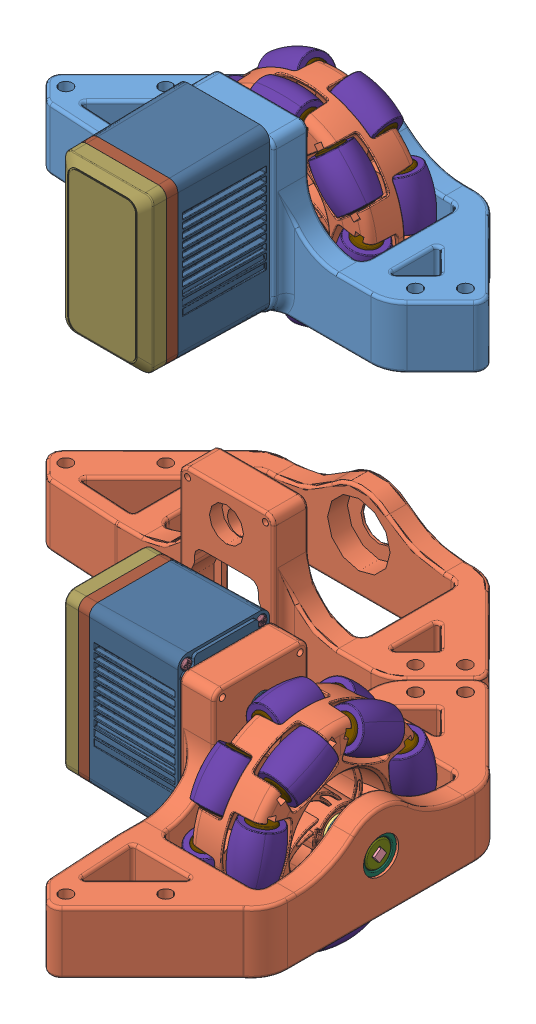
SolidWorks assembly holo_bracket_v4_Front_testfit, configuration Default. Lengths in mm.
Overall size (299.11 89.8 299.11).
176 component instances, 23 part files, 31 mates.
Components (placement in the parent):
- holo_bracket_v4_Left-1: holo_bracket_v4_Left [Default] at (46.7387 84.3688 112.9136) size (147.75 57.17 55.6)
- holo_bracket_v4_Right-1: holo_bracket_v4_Right [Default] at (163.9131 84.3688 230.088) size (181.94 57.17 181.94)
- V5 Smart Motor (276-4840) no cap-1: V5 Smart Motor (276-4840) no cap [Default] at (195.0559 116.1188 308.4808) x (0 -1 0) z (1 0 0) size (59.01 35.33 59.91)
  - V5 Smart Motor (276-4840).step-1: V5 Smart Motor (276-4840).step [Default] at origin size (59.01 35.33 59.91)
    - 276-4840-900 Rev6_Instruction.step-1: 276-4840-900 Rev6_Instruction.step [Default] at (-14.3 0 -17.2) size (52.79 15.94 38.15)
      - 276-4840-901 Rev6.step-1: 276-4840-901 Rev6.step [Default] at (10.75 -10.05 17.8) x (-1 0 0) z (0 0 1) size (49.9 1.6 38.15)
      - 276-4840-902 Rev2.step-1: 276-4840-902 Rev2.step [Default] at (31.25 -9.25 6.2) x (0 0 -1) z (0 -1 0) size (10.35 11.39 15.94)
      - 276-4840-022 Rev4.step-1: 276-4840-022 Rev4.step [Default] at (31.25 -9.25 6.2) x (0 0 -1) z (1 0 0) size (10.26 9.1 5.51)
    - 276-4840-110 Rev10_Instruction.step-1: 276-4840-110 Rev10_Instruction.step [Default] at (12.7 0 14.7) size (35.33 35.33 31.1)
      - 276-4840-061 Rev7_Ring_Gear_Fixed01 .6 Rev3.step-1: 276-4840-061 Rev7_Ring_Gear_Fixed01 .6 Rev3.step [Default] at origin size (28.79 28.39 24.6)
      - 276-4840-018 Rev6.step-1: 276-4840-018 Rev6.step [Default] at (0 0 6.7) x (-0.483174 0.875524 0) z (0 0 1) size (26 26 12.3)
      - 276-4840-059 Rev2.step-1: 276-4840-059 Rev2.step [Default] at (0 0 10.3) size (28.4 28.4 8.5)
      - 276-4840-062 Rev1.step-1: 276-4840-062 Rev1.step [Default] at (-12.1353 8.8168 12.3) x (0.956835 -0.290632 0) z (-0.290632 -0.956835 0) size (3.2 6.56 3.2)
      - 276-4840-062 Rev1.step-2: 276-4840-062 Rev1.step [Default] at (12.1353 8.8168 12.3) x (0.978427 0.206591 0) z (0.206591 -0.978427 0) size (3.2 6.56 3.2)
      - 276-4840-062 Rev1.step-3: 276-4840-062 Rev1.step [Default] at (-12.1353 -8.8168 12.3) x (0.72563 0.688086 0) z (0.688086 -0.72563 0) size (3.2 6.56 3.2)
    - 276-4840-001 Rev38.step-1: 276-4840-001 Rev38.step [Default] at origin size (57.3 33 46.9)
    - 276-4840-005 Rev27.step-1: 276-4840-005 Rev27.step [Default] at (0 0 -17.95) size (56.17 31.87 12.9)
    - 276-4840-004 Rev16.step-1: 276-4840-004 Rev16.step [Default] at (0 0 -19.2) size (56.01 31.71 9.21)
    - 276-4840-009 Rev3.step-1: 276-4840-009 Rev3.step [Default] at (25.45 13.5 15.7) x (0.19987 -0.979823 0) z (-0.979823 -0.19987 0) size (3.4 41.31 4.34)
    - 276-4840-009 Rev3.step-2: 276-4840-009 Rev3.step [Default] at (-25.45 -13.5 15.7) x (-0.998855 0.047836 0) z (0.047836 0.998855 0) size (3.4 41.31 4.34)
    - 276-4840-009 Rev3.step-3: 276-4840-009 Rev3.step [Default] at (25.45 -13.5 15.7) x (-0.975374 0.220559 0) z (0.220559 0.975374 0) size (3.4 41.31 4.34)
    - 276-4840-009 Rev3.step-4: 276-4840-009 Rev3.step [Default] at (-25.45 13.5 15.7) x (-0.922256 0.38658 0) z (0.38658 0.922256 0) size (3.4 41.31 4.34)
    - 276-4840-025 Rev19.step-1: 276-4840-025 Rev19.step [Default] at (12.7 0 -22.63) x (-0.993315 0.115437 0) z (0 0 1) size (14.82 14.83 35.18)
- V5 Smart Motor (276-4840) no cap-2: V5 Smart Motor (276-4840) no cap [Default] at (46.7387 116.1188 160.1636) x (0 -1 0) z (0 0 -1) size (59.01 35.33 59.91)
  - V5 Smart Motor (276-4840).step-1: V5 Smart Motor (276-4840).step [Default] at origin size (59.01 35.33 59.91)
    - 276-4840-900 Rev6_Instruction.step-1: 276-4840-900 Rev6_Instruction.step [Default] at (-14.3 0 -17.2) size (52.79 15.94 38.15)
      - 276-4840-901 Rev6.step-1: 276-4840-901 Rev6.step [Default] at (10.75 -10.05 17.8) x (-1 0 0) z (0 0 1) size (49.9 1.6 38.15)
      - 276-4840-902 Rev2.step-1: 276-4840-902 Rev2.step [Default] at (31.25 -9.25 6.2) x (0 0 -1) z (0 -1 0) size (10.35 11.39 15.94)
      - 276-4840-022 Rev4.step-1: 276-4840-022 Rev4.step [Default] at (31.25 -9.25 6.2) x (0 0 -1) z (1 0 0) size (10.26 9.1 5.51)
    - 276-4840-110 Rev10_Instruction.step-1: 276-4840-110 Rev10_Instruction.step [Default] at (12.7 0 14.7) size (35.33 35.33 31.1)
      - 276-4840-061 Rev7_Ring_Gear_Fixed01 .6 Rev3.step-1: 276-4840-061 Rev7_Ring_Gear_Fixed01 .6 Rev3.step [Default] at origin size (28.79 28.39 24.6)
      - 276-4840-018 Rev6.step-1: 276-4840-018 Rev6.step [Default] at (0 0 6.7) x (-0.483174 0.875524 0) z (0 0 1) size (26 26 12.3)
      - 276-4840-059 Rev2.step-1: 276-4840-059 Rev2.step [Default] at (0 0 10.3) size (28.4 28.4 8.5)
      - 276-4840-062 Rev1.step-1: 276-4840-062 Rev1.step [Default] at (-12.1353 8.8168 12.3) x (0.956835 -0.290632 0) z (-0.290632 -0.956835 0) size (3.2 6.56 3.2)
      - 276-4840-062 Rev1.step-2: 276-4840-062 Rev1.step [Default] at (12.1353 8.8168 12.3) x (0.978427 0.206591 0) z (0.206591 -0.978427 0) size (3.2 6.56 3.2)
      - 276-4840-062 Rev1.step-3: 276-4840-062 Rev1.step [Default] at (-12.1353 -8.8168 12.3) x (0.72563 0.688086 0) z (0.688086 -0.72563 0) size (3.2 6.56 3.2)
    - 276-4840-001 Rev38.step-1: 276-4840-001 Rev38.step [Default] at origin size (57.3 33 46.9)
    - 276-4840-005 Rev27.step-1: 276-4840-005 Rev27.step [Default] at (0 0 -17.95) size (56.17 31.87 12.9)
    - 276-4840-004 Rev16.step-1: 276-4840-004 Rev16.step [Default] at (0 0 -19.2) size (56.01 31.71 9.21)
    - 276-4840-009 Rev3.step-1: 276-4840-009 Rev3.step [Default] at (25.45 13.5 15.7) x (0.19987 -0.979823 0) z (-0.979823 -0.19987 0) size (3.4 41.31 4.34)
    - 276-4840-009 Rev3.step-2: 276-4840-009 Rev3.step [Default] at (-25.45 -13.5 15.7) x (-0.998855 0.047836 0) z (0.047836 0.998855 0) size (3.4 41.31 4.34)
    - 276-4840-009 Rev3.step-3: 276-4840-009 Rev3.step [Default] at (25.45 -13.5 15.7) x (-0.975374 0.220559 0) z (0.220559 0.975374 0) size (3.4 41.31 4.34)
    - 276-4840-009 Rev3.step-4: 276-4840-009 Rev3.step [Default] at (-25.45 13.5 15.7) x (-0.922256 0.38658 0) z (0.38658 0.922256 0) size (3.4 41.31 4.34)
    - 276-4840-025 Rev19.step-1: 276-4840-025 Rev19.step [Default] at (12.7 0 -22.63) x (-0.993315 0.115437 0) z (0 0 1) size (14.82 14.83 35.18)
- 0.375_ ID x 0.875_ OD x 0.281_ WD (Radial Bearing) (217-3239)-1: 0.375_ ID x 0.875_ OD x 0.281_ WD (Radial Bearing) (217-3239) [Default] at (259.8559 103.4188 308.4808) size (7.14 22.23 22.23)
- 0.375_ ID x 0.875_ OD x 0.281_ WD (Radial Bearing) (217-3239)-2: 0.375_ ID x 0.875_ OD x 0.281_ WD (Radial Bearing) (217-3239) [Default] at (46.7387 103.4188 88.2262) x (0 0 1) z (-1 0 0) size (7.14 22.23 22.23)
- 0.375in_ID_Bearing_Insert-1: 0.375in_ID_Bearing_Insert [Default] at (266.9999 103.4188 308.4808) x (0 0.801872 0.597496) z (-1 0 0) size (9.4 9.4 7.14)
- 0.375in_ID_Bearing_Insert-2: 0.375in_ID_Bearing_Insert [Default] at (46.7387 103.4188 95.3702) x (-0.877149 0.480218 0) z (0 0 -1) size (9.4 9.4 7.14)
- 2.75 Omni with inserts (276-1902) -1: 2.75 Omni with inserts (276-1902)  [Default] at (310.5892 53.5782 282.6771) x (0 0 1) z (-1 0 0) size (87.15 87.98 47.75)
  - 2.75 Omni-Directional Wheel - Double Roller (276-1902) -1: 2.75 Omni-Directional Wheel - Double Roller (276-1902)  [Default] at (25.8037 49.8406 68.5807) size (87.15 87.98 47.75)
    - 2.75 Omni-Directional Wheel - Double Roller (276-1902) .step-1: 2.75 Omni-Directional Wheel - Double Roller (276-1902) .step [Default] at origin size (87.15 87.98 47.75)
      - 276-1902-010 Rev1.step-1: 276-1902-010 Rev1.step [Default] at (0 27.5 8) x (1 0 0) z (0 0.828233 0.560383) size (23 27.81 20.35)
        - 276-1902-011 Rev1.step-1: 276-1902-011 Rev1.step [Default] at (0 -6.325 -26.7627) x (1 0 0) z (0 -0.973191 0.23) size (16.5 15 25.03)
        - 276-1902-012 Rev1.step-1: 276-1902-012 Rev1.step [Default] at origin size (17.5 10.34 18.34)
        - 276-1902-003 Rev1.step-1: 276-1902-003 Rev1.step [Default] x (0 -0.928523 0.371275) z (1 0 0) size (2 2 23)
      - 276-1902-010 Rev1.step-2: 276-1902-010 Rev1.step [Default] at (0 -27.5 -8) x (1 0 0) z (0 0.410464 0.911877) size (23 27.81 20.35)
        - 276-1902-011 Rev1.step-1: 276-1902-011 Rev1.step [Default] at (0 -6.325 -26.7627) x (1 0 0) z (0 -0.973191 0.23) size (16.5 15 25.03)
        - 276-1902-012 Rev1.step-1: 276-1902-012 Rev1.step [Default] at origin size (17.5 10.34 18.34)
        - 276-1902-003 Rev1.step-1: 276-1902-003 Rev1.step [Default] x (0 -0.928523 0.371275) z (1 0 0) size (2 2 23)
      - 276-1902-010 Rev1.step-3: 276-1902-010 Rev1.step [Default] at (-21.5004 -17.146 -8) x (0.62349 -0.781831 0) z (0.320913 0.25592 0.911877) size (23 27.81 20.35)
        - 276-1902-011 Rev1.step-1: 276-1902-011 Rev1.step [Default] at (0 -6.325 -26.7627) x (1 0 0) z (0 -0.973191 0.23) size (16.5 15 25.03)
        - 276-1902-012 Rev1.step-1: 276-1902-012 Rev1.step [Default] at origin size (17.5 10.34 18.34)
        - 276-1902-003 Rev1.step-1: 276-1902-003 Rev1.step [Default] x (0 -0.928523 0.371275) z (1 0 0) size (2 2 23)
      - 276-1902-010 Rev1.step-4: 276-1902-010 Rev1.step [Default] at (-26.8105 6.1193 -8) x (-0.222521 -0.974928 0) z (0.400172 -0.091337 0.911877) size (23 27.81 20.35)
        - 276-1902-011 Rev1.step-1: 276-1902-011 Rev1.step [Default] at (0 -6.325 -26.7627) x (1 0 0) z (0 -0.973191 0.23) size (16.5 15 25.03)
        - 276-1902-012 Rev1.step-1: 276-1902-012 Rev1.step [Default] at origin size (17.5 10.34 18.34)
        - 276-1902-003 Rev1.step-1: 276-1902-003 Rev1.step [Default] x (0 -0.928523 0.371275) z (1 0 0) size (2 2 23)
      - 276-1902-010 Rev1.step-5: 276-1902-010 Rev1.step [Default] at (-11.9318 24.7766 -8) x (-0.900969 -0.433884 0) z (0.178093 -0.369815 0.911877) size (23 27.81 20.35)
        - 276-1902-011 Rev1.step-1: 276-1902-011 Rev1.step [Default] at (0 -6.325 -26.7627) x (1 0 0) z (0 -0.973191 0.23) size (16.5 15 25.03)
        - 276-1902-012 Rev1.step-1: 276-1902-012 Rev1.step [Default] at origin size (17.5 10.34 18.34)
        - 276-1902-003 Rev1.step-1: 276-1902-003 Rev1.step [Default] x (0 -0.928523 0.371275) z (1 0 0) size (2 2 23)
      - 276-1902-010 Rev1.step-6: 276-1902-010 Rev1.step [Default] at (11.9318 24.7766 -8) x (-0.900969 0.433884 0) z (-0.178093 -0.369815 0.911877) size (23 27.81 20.35)
        - 276-1902-011 Rev1.step-1: 276-1902-011 Rev1.step [Default] at (0 -6.325 -26.7627) x (1 0 0) z (0 -0.973191 0.23) size (16.5 15 25.03)
        - 276-1902-012 Rev1.step-1: 276-1902-012 Rev1.step [Default] at origin size (17.5 10.34 18.34)
        - 276-1902-003 Rev1.step-1: 276-1902-003 Rev1.step [Default] x (0 -0.928523 0.371275) z (1 0 0) size (2 2 23)
      - 276-1902-010 Rev1.step-7: 276-1902-010 Rev1.step [Default] at (26.8105 6.1193 -8) x (-0.222521 0.974928 0) z (-0.400172 -0.091337 0.911877) size (23 27.81 20.35)
        - 276-1902-011 Rev1.step-1: 276-1902-011 Rev1.step [Default] at (0 -6.325 -26.7627) x (1 0 0) z (0 -0.973191 0.23) size (16.5 15 25.03)
        - 276-1902-012 Rev1.step-1: 276-1902-012 Rev1.step [Default] at origin size (17.5 10.34 18.34)
        - 276-1902-003 Rev1.step-1: 276-1902-003 Rev1.step [Default] x (0 -0.928523 0.371275) z (1 0 0) size (2 2 23)
      - 276-1902-010 Rev1.step-8: 276-1902-010 Rev1.step [Default] at (21.5004 -17.146 -8) x (0.62349 0.781831 0) z (-0.320913 0.25592 0.911877) size (23 27.81 20.35)
        - 276-1902-011 Rev1.step-1: 276-1902-011 Rev1.step [Default] at (0 -6.325 -26.7627) x (1 0 0) z (0 -0.973191 0.23) size (16.5 15 25.03)
        - 276-1902-012 Rev1.step-1: 276-1902-012 Rev1.step [Default] at origin size (17.5 10.34 18.34)
        - 276-1902-003 Rev1.step-1: 276-1902-003 Rev1.step [Default] x (0 -0.928523 0.371275) z (1 0 0) size (2 2 23)
      - 276-1902-010 Rev1.step-9: 276-1902-010 Rev1.step [Default] at (21.5004 17.146 8) x (0.62349 -0.781831 0) z (0.647539 0.516395 0.560383) size (23 27.81 20.35)
        - 276-1902-011 Rev1.step-1: 276-1902-011 Rev1.step [Default] at (0 -6.325 -26.7627) x (1 0 0) z (0 -0.973191 0.23) size (16.5 15 25.03)
        - 276-1902-012 Rev1.step-1: 276-1902-012 Rev1.step [Default] at origin size (17.5 10.34 18.34)
        - 276-1902-003 Rev1.step-1: 276-1902-003 Rev1.step [Default] x (0 -0.928523 0.371275) z (1 0 0) size (2 2 23)
      - 276-1902-010 Rev1.step-10: 276-1902-010 Rev1.step [Default] at (26.8105 -6.1193 8) x (-0.222521 -0.974928 0) z (0.807468 -0.184299 0.560383) size (23 27.81 20.35)
        - 276-1902-011 Rev1.step-1: 276-1902-011 Rev1.step [Default] at (0 -6.325 -26.7627) x (1 0 0) z (0 -0.973191 0.23) size (16.5 15 25.03)
        - 276-1902-012 Rev1.step-1: 276-1902-012 Rev1.step [Default] at origin size (17.5 10.34 18.34)
        - 276-1902-003 Rev1.step-1: 276-1902-003 Rev1.step [Default] x (0 -0.928523 0.371275) z (1 0 0) size (2 2 23)
      - 276-1902-010 Rev1.step-11: 276-1902-010 Rev1.step [Default] at (11.9318 -24.7766 8) x (-0.900969 -0.433884 0) z (0.359357 -0.746212 0.560383) size (23 27.81 20.35)
        - 276-1902-011 Rev1.step-1: 276-1902-011 Rev1.step [Default] at (0 -6.325 -26.7627) x (1 0 0) z (0 -0.973191 0.23) size (16.5 15 25.03)
        - 276-1902-012 Rev1.step-1: 276-1902-012 Rev1.step [Default] at origin size (17.5 10.34 18.34)
        - 276-1902-003 Rev1.step-1: 276-1902-003 Rev1.step [Default] x (0 -0.928523 0.371275) z (1 0 0) size (2 2 23)
      - 276-1902-010 Rev1.step-12: 276-1902-010 Rev1.step [Default] at (-11.9318 -24.7766 8) x (-0.900969 0.433884 0) z (-0.359357 -0.746212 0.560383) size (23 27.81 20.35)
        - 276-1902-011 Rev1.step-1: 276-1902-011 Rev1.step [Default] at (0 -6.325 -26.7627) x (1 0 0) z (0 -0.973191 0.23) size (16.5 15 25.03)
        - 276-1902-012 Rev1.step-1: 276-1902-012 Rev1.step [Default] at origin size (17.5 10.34 18.34)
        - 276-1902-003 Rev1.step-1: 276-1902-003 Rev1.step [Default] x (0 -0.928523 0.371275) z (1 0 0) size (2 2 23)
      - 276-1902-010 Rev1.step-13: 276-1902-010 Rev1.step [Default] at (-26.8105 -6.1193 8) x (-0.222521 0.974928 0) z (-0.807468 -0.184299 0.560383) size (23 27.81 20.35)
        - 276-1902-011 Rev1.step-1: 276-1902-011 Rev1.step [Default] at (0 -6.325 -26.7627) x (1 0 0) z (0 -0.973191 0.23) size (16.5 15 25.03)
        - 276-1902-012 Rev1.step-1: 276-1902-012 Rev1.step [Default] at origin size (17.5 10.34 18.34)
        - 276-1902-003 Rev1.step-1: 276-1902-003 Rev1.step [Default] x (0 -0.928523 0.371275) z (1 0 0) size (2 2 23)
      - 276-1902-010 Rev1.step-14: 276-1902-010 Rev1.step [Default] at (-21.5004 17.146 8) x (0.62349 0.781831 0) z (-0.647539 0.516395 0.560383) size (23 27.81 20.35)
        - 276-1902-011 Rev1.step-1: 276-1902-011 Rev1.step [Default] at (0 -6.325 -26.7627) x (1 0 0) z (0 -0.973191 0.23) size (16.5 15 25.03)
        - 276-1902-012 Rev1.step-1: 276-1902-012 Rev1.step [Default] at origin size (17.5 10.34 18.34)
        - 276-1902-003 Rev1.step-1: 276-1902-003 Rev1.step [Default] x (0 -0.928523 0.371275) z (1 0 0) size (2 2 23)
      - 276-1902-002 Rev3.step-1: 276-1902-002 Rev3.step [Default] at origin size (66.55 66.02 25.07)
  - Metal Shaft Inserts (276-3881-002)-1: Metal Shaft Inserts (276-3881-002) [Default] at (25.8037 49.8406 79.8307) x (0 -1 0) z (1 0 0) size (10.03 5.08 10.03)
  - Metal Shaft Inserts (276-3881-002)-2: Metal Shaft Inserts (276-3881-002) [Default] at (25.8037 49.8406 57.3307) x (1 0 0) z (0 -1 0) size (10.03 5.08 10.03)
- 2.75 Omni with inserts (276-1902) -2: 2.75 Omni with inserts (276-1902)  [Default] at (21.9935 53.0443 44.6435) x (0.999777 0.021121 0) z (0 0 1) size (87.15 87.98 47.75)
  - 2.75 Omni-Directional Wheel - Double Roller (276-1902) -1: 2.75 Omni-Directional Wheel - Double Roller (276-1902)  [Default] at (25.8037 49.8406 68.5807) size (87.15 87.98 47.75)
    - 2.75 Omni-Directional Wheel - Double Roller (276-1902) .step-1: 2.75 Omni-Directional Wheel - Double Roller (276-1902) .step [Default] at origin size (87.15 87.98 47.75)
      - 276-1902-010 Rev1.step-1: 276-1902-010 Rev1.step [Default] at (0 27.5 8) x (1 0 0) z (0 0.828233 0.560383) size (23 27.81 20.35)
        - 276-1902-011 Rev1.step-1: 276-1902-011 Rev1.step [Default] at (0 -6.325 -26.7627) x (1 0 0) z (0 -0.973191 0.23) size (16.5 15 25.03)
        - 276-1902-012 Rev1.step-1: 276-1902-012 Rev1.step [Default] at origin size (17.5 10.34 18.34)
        - 276-1902-003 Rev1.step-1: 276-1902-003 Rev1.step [Default] x (0 -0.928523 0.371275) z (1 0 0) size (2 2 23)
      - 276-1902-010 Rev1.step-2: 276-1902-010 Rev1.step [Default] at (0 -27.5 -8) x (1 0 0) z (0 0.410464 0.911877) size (23 27.81 20.35)
        - 276-1902-011 Rev1.step-1: 276-1902-011 Rev1.step [Default] at (0 -6.325 -26.7627) x (1 0 0) z (0 -0.973191 0.23) size (16.5 15 25.03)
        - 276-1902-012 Rev1.step-1: 276-1902-012 Rev1.step [Default] at origin size (17.5 10.34 18.34)
        - 276-1902-003 Rev1.step-1: 276-1902-003 Rev1.step [Default] x (0 -0.928523 0.371275) z (1 0 0) size (2 2 23)
      - 276-1902-010 Rev1.step-3: 276-1902-010 Rev1.step [Default] at (-21.5004 -17.146 -8) x (0.62349 -0.781831 0) z (0.320913 0.25592 0.911877) size (23 27.81 20.35)
        - 276-1902-011 Rev1.step-1: 276-1902-011 Rev1.step [Default] at (0 -6.325 -26.7627) x (1 0 0) z (0 -0.973191 0.23) size (16.5 15 25.03)
        - 276-1902-012 Rev1.step-1: 276-1902-012 Rev1.step [Default] at origin size (17.5 10.34 18.34)
        - 276-1902-003 Rev1.step-1: 276-1902-003 Rev1.step [Default] x (0 -0.928523 0.371275) z (1 0 0) size (2 2 23)
      - 276-1902-010 Rev1.step-4: 276-1902-010 Rev1.step [Default] at (-26.8105 6.1193 -8) x (-0.222521 -0.974928 0) z (0.400172 -0.091337 0.911877) size (23 27.81 20.35)
        - 276-1902-011 Rev1.step-1: 276-1902-011 Rev1.step [Default] at (0 -6.325 -26.7627) x (1 0 0) z (0 -0.973191 0.23) size (16.5 15 25.03)
        - 276-1902-012 Rev1.step-1: 276-1902-012 Rev1.step [Default] at origin size (17.5 10.34 18.34)
        - 276-1902-003 Rev1.step-1: 276-1902-003 Rev1.step [Default] x (0 -0.928523 0.371275) z (1 0 0) size (2 2 23)
      - 276-1902-010 Rev1.step-5: 276-1902-010 Rev1.step [Default] at (-11.9318 24.7766 -8) x (-0.900969 -0.433884 0) z (0.178093 -0.369815 0.911877) size (23 27.81 20.35)
        - 276-1902-011 Rev1.step-1: 276-1902-011 Rev1.step [Default] at (0 -6.325 -26.7627) x (1 0 0) z (0 -0.973191 0.23) size (16.5 15 25.03)
        - 276-1902-012 Rev1.step-1: 276-1902-012 Rev1.step [Default] at origin size (17.5 10.34 18.34)
        - 276-1902-003 Rev1.step-1: 276-1902-003 Rev1.step [Default] x (0 -0.928523 0.371275) z (1 0 0) size (2 2 23)
      - 276-1902-010 Rev1.step-6: 276-1902-010 Rev1.step [Default] at (11.9318 24.7766 -8) x (-0.900969 0.433884 0) z (-0.178093 -0.369815 0.911877) size (23 27.81 20.35)
        - 276-1902-011 Rev1.step-1: 276-1902-011 Rev1.step [Default] at (0 -6.325 -26.7627) x (1 0 0) z (0 -0.973191 0.23) size (16.5 15 25.03)
        - 276-1902-012 Rev1.step-1: 276-1902-012 Rev1.step [Default] at origin size (17.5 10.34 18.34)
        - 276-1902-003 Rev1.step-1: 276-1902-003 Rev1.step [Default] x (0 -0.928523 0.371275) z (1 0 0) size (2 2 23)
      - 276-1902-010 Rev1.step-7: 276-1902-010 Rev1.step [Default] at (26.8105 6.1193 -8) x (-0.222521 0.974928 0) z (-0.400172 -0.091337 0.911877) size (23 27.81 20.35)
        - 276-1902-011 Rev1.step-1: 276-1902-011 Rev1.step [Default] at (0 -6.325 -26.7627) x (1 0 0) z (0 -0.973191 0.23) size (16.5 15 25.03)
        - 276-1902-012 Rev1.step-1: 276-1902-012 Rev1.step [Default] at origin size (17.5 10.34 18.34)
        - 276-1902-003 Rev1.step-1: 276-1902-003 Rev1.step [Default] x (0 -0.928523 0.371275) z (1 0 0) size (2 2 23)
      - 276-1902-010 Rev1.step-8: 276-1902-010 Rev1.step [Default] at (21.5004 -17.146 -8) x (0.62349 0.781831 0) z (-0.320913 0.25592 0.911877) size (23 27.81 20.35)
        - 276-1902-011 Rev1.step-1: 276-1902-011 Rev1.step [Default] at (0 -6.325 -26.7627) x (1 0 0) z (0 -0.973191 0.23) size (16.5 15 25.03)
        - 276-1902-012 Rev1.step-1: 276-1902-012 Rev1.step [Default] at origin size (17.5 10.34 18.34)
        - 276-1902-003 Rev1.step-1: 276-1902-003 Rev1.step [Default] x (0 -0.928523 0.371275) z (1 0 0) size (2 2 23)
      - 276-1902-010 Rev1.step-9: 276-1902-010 Rev1.step [Default] at (21.5004 17.146 8) x (0.62349 -0.781831 0) z (0.647539 0.516395 0.560383) size (23 27.81 20.35)
        - 276-1902-011 Rev1.step-1: 276-1902-011 Rev1.step [Default] at (0 -6.325 -26.7627) x (1 0 0) z (0 -0.973191 0.23) size (16.5 15 25.03)
        - 276-1902-012 Rev1.step-1: 276-1902-012 Rev1.step [Default] at origin size (17.5 10.34 18.34)
        - 276-1902-003 Rev1.step-1: 276-1902-003 Rev1.step [Default] x (0 -0.928523 0.371275) z (1 0 0) size (2 2 23)
      - 276-1902-010 Rev1.step-10: 276-1902-010 Rev1.step [Default] at (26.8105 -6.1193 8) x (-0.222521 -0.974928 0) z (0.807468 -0.184299 0.560383) size (23 27.81 20.35)
        - 276-1902-011 Rev1.step-1: 276-1902-011 Rev1.step [Default] at (0 -6.325 -26.7627) x (1 0 0) z (0 -0.973191 0.23) size (16.5 15 25.03)
        - 276-1902-012 Rev1.step-1: 276-1902-012 Rev1.step [Default] at origin size (17.5 10.34 18.34)
        - 276-1902-003 Rev1.step-1: 276-1902-003 Rev1.step [Default] x (0 -0.928523 0.371275) z (1 0 0) size (2 2 23)
      - 276-1902-010 Rev1.step-11: 276-1902-010 Rev1.step [Default] at (11.9318 -24.7766 8) x (-0.900969 -0.433884 0) z (0.359357 -0.746212 0.560383) size (23 27.81 20.35)
        - 276-1902-011 Rev1.step-1: 276-1902-011 Rev1.step [Default] at (0 -6.325 -26.7627) x (1 0 0) z (0 -0.973191 0.23) size (16.5 15 25.03)
        - 276-1902-012 Rev1.step-1: 276-1902-012 Rev1.step [Default] at origin size (17.5 10.34 18.34)
        - 276-1902-003 Rev1.step-1: 276-1902-003 Rev1.step [Default] x (0 -0.928523 0.371275) z (1 0 0) size (2 2 23)
      - 276-1902-010 Rev1.step-12: 276-1902-010 Rev1.step [Default] at (-11.9318 -24.7766 8) x (-0.900969 0.433884 0) z (-0.359357 -0.746212 0.560383) size (23 27.81 20.35)
        - 276-1902-011 Rev1.step-1: 276-1902-011 Rev1.step [Default] at (0 -6.325 -26.7627) x (1 0 0) z (0 -0.973191 0.23) size (16.5 15 25.03)
        - 276-1902-012 Rev1.step-1: 276-1902-012 Rev1.step [Default] at origin size (17.5 10.34 18.34)
        - 276-1902-003 Rev1.step-1: 276-1902-003 Rev1.step [Default] x (0 -0.928523 0.371275) z (1 0 0) size (2 2 23)
      - 276-1902-010 Rev1.step-13: 276-1902-010 Rev1.step [Default] at (-26.8105 -6.1193 8) x (-0.222521 0.974928 0) z (-0.807468 -0.184299 0.560383) size (23 27.81 20.35)
        - 276-1902-011 Rev1.step-1: 276-1902-011 Rev1.step [Default] at (0 -6.325 -26.7627) x (1 0 0) z (0 -0.973191 0.23) size (16.5 15 25.03)
        - 276-1902-012 Rev1.step-1: 276-1902-012 Rev1.step [Default] at origin size (17.5 10.34 18.34)
        - 276-1902-003 Rev1.step-1: 276-1902-003 Rev1.step [Default] x (0 -0.928523 0.371275) z (1 0 0) size (2 2 23)
      - 276-1902-010 Rev1.step-14: 276-1902-010 Rev1.step [Default] at (-21.5004 17.146 8) x (0.62349 0.781831 0) z (-0.647539 0.516395 0.560383) size (23 27.81 20.35)
        - 276-1902-011 Rev1.step-1: 276-1902-011 Rev1.step [Default] at (0 -6.325 -26.7627) x (1 0 0) z (0 -0.973191 0.23) size (16.5 15 25.03)
        - 276-1902-012 Rev1.step-1: 276-1902-012 Rev1.step [Default] at origin size (17.5 10.34 18.34)
        - 276-1902-003 Rev1.step-1: 276-1902-003 Rev1.step [Default] x (0 -0.928523 0.371275) z (1 0 0) size (2 2 23)
      - 276-1902-002 Rev3.step-1: 276-1902-002 Rev3.step [Default] at origin size (66.55 66.02 25.07)
  - Metal Shaft Inserts (276-3881-002)-1: Metal Shaft Inserts (276-3881-002) [Default] at (25.8037 49.8406 79.8307) x (0 -1 0) z (1 0 0) size (10.03 5.08 10.03)
  - Metal Shaft Inserts (276-3881-002)-2: Metal Shaft Inserts (276-3881-002) [Default] at (25.8037 49.8406 57.3307) x (1 0 0) z (0 -1 0) size (10.03 5.08 10.03)
- Drive Shaft 2in-1: Drive Shaft 2in [Default] at (369.2559 103.4188 308.4808) x (0 0.801872 0.597496) z (-1 0 0) size (3.28 3.28 50.8)
- Drive Shaft 2in-2: Drive Shaft 2in [Default] at (46.7387 103.4188 -14.0364) x (-0.480218 -0.877149 0) z (0 0 1) size (3.28 3.28 50.8)
- Shaft Collar (276-2010)-1: Shaft Collar (276-2010) [Default] at (256.5605 103.4188 308.4808) x (0 0 1) z (-1 0 0) size (11 11.35 6.6)
- Shaft Collar (276-2010)-2: Shaft Collar (276-2010) [Default] at (46.7387 103.4188 98.6722) size (11 11.35 6.6)
Mates (geometry in assembly coordinates):
- Coincident1: coincident aligned: plane of holo_bracket_v4_Left-1 through (78.9533 106.6188 80.699) normal (0.707107 0 -0.707107); plane of holo_bracket_v4_Right-1 through (274.5205 106.6188 276.2662) normal (0.707107 0 -0.707107)
- Coincident2: coincident aligned: plane of holo_bracket_v4_Left-1 through (46.7387 106.6188 112.9136) normal (0 1 0); plane of holo_bracket_v4_Right-1 through (242.3059 106.6188 308.4808) normal (0 1 0)
- Distance1: distance = 355.6 mm: cylinder of holo_bracket_v4_Left-1 through (-7.1428 106.6188 110.9152) axis (0 -1 0) radius 2.3; cylinder of holo_bracket_v4_Right-1 through (244.3044 106.6188 362.3623) axis (0 -1 0) radius 2.3
- Coincident4: coincident anti-aligned: plane of holo_bracket_v4_Right-1 through (212.2559 84.3688 308.4808) normal (-1 0 0); plane of V5 Smart Motor (276-4840) no cap-1/V5 Smart Motor (276-4840).step-1/276-4840-001 Rev38.step-1 through (212.2559 141.1688 295.5808) normal (1 0 0)
- Concentric2: concentric aligned: cylinder of holo_bracket_v4_Right-1 through (267.8569 103.4188 308.4808) axis (-1 0 0) radius 14.5; cone of V5 Smart Motor (276-4840) no cap-1/V5 Smart Motor (276-4840).step-1/276-4840-110 Rev10_Instruction.step-1/276-4840-061 Rev7_Ring_Gear_Fixed01 .6 Rev3.step-1 through (197.4559 103.4188 308.4808) axis (-1 0 0)
- Parallel1: parallel anti-aligned: line of holo_bracket_v4_Right-1 through (213.2559 141.0688 322.4808) axis (0 0 -1); line of V5 Smart Motor (276-4840) no cap-1/V5 Smart Motor (276-4840).step-1/276-4840-001 Rev38.step-1 through (211.2559 144.7688 295.5808) axis (0 0 1)
- Coincident6: coincident anti-aligned: plane of holo_bracket_v4_Left-1 through (46.7387 84.3688 142.9636) normal (0 0 1); plane of V5 Smart Motor (276-4840) no cap-2/V5 Smart Motor (276-4840).step-1/276-4840-001 Rev38.step-1 through (33.8387 141.1688 142.9636) normal (0 0 -1)
- Concentric3: concentric aligned: cylinder of holo_bracket_v4_Left-1 through (46.7387 103.4188 87.3626) axis (0 0 1) radius 14.5; cone of V5 Smart Motor (276-4840) no cap-2/V5 Smart Motor (276-4840).step-1/276-4840-110 Rev10_Instruction.step-1/276-4840-061 Rev7_Ring_Gear_Fixed01 .6 Rev3.step-1 through (46.7387 103.4188 157.7636) axis (0 0 1)
- Parallel2: parallel anti-aligned: line of holo_bracket_v4_Left-1 through (60.7387 141.0688 131.4636) axis (-1 0 0); line of V5 Smart Motor (276-4840) no cap-2/V5 Smart Motor (276-4840).step-1/276-4840-001 Rev38.step-1 through (33.8387 144.7688 143.9636) axis (1 0 0)
- Concentric4: concentric anti-aligned: cylinder of 0.375_ ID x 0.875_ OD x 0.281_ WD (Radial Bearing) (217-3239)-1 through (245.319 103.4188 308.4808) axis (-1 0 0) radius 4.763; cylinder of 0.375in_ID_Bearing_Insert-1 through (259.8625 103.4188 308.4808) axis (1 0 0) radius 4.7
- Coincident8: coincident aligned: plane of 0.375_ ID x 0.875_ OD x 0.281_ WD (Radial Bearing) (217-3239)-1 through (266.9999 97.0518 308.4808) normal (1 0 0); plane of 0.375in_ID_Bearing_Insert-1 through (266.9999 103.4188 308.4808) normal (1 0 0)
- Concentric5: concentric anti-aligned: cylinder of 0.375_ ID x 0.875_ OD x 0.281_ WD (Radial Bearing) (217-3239)-2 through (46.7387 103.4188 73.6893) axis (0 0 -1) radius 4.763; cylinder of 0.375in_ID_Bearing_Insert-2 through (46.7387 103.4188 88.2328) axis (0 0 1) radius 4.7
- Coincident9: coincident aligned: plane of 0.375_ ID x 0.875_ OD x 0.281_ WD (Radial Bearing) (217-3239)-2 through (46.7387 97.0518 95.3702) normal (0 0 1); plane of 0.375in_ID_Bearing_Insert-2 through (46.7387 103.4188 95.3702) normal (0 0 1)
- Concentric6: concentric anti-aligned: cylinder of holo_bracket_v4_Left-1 through (46.7387 103.4188 88.2262) axis (0 0 1) radius 11.25; cylinder of 0.375_ ID x 0.875_ OD x 0.281_ WD (Radial Bearing) (217-3239)-2 through (46.7387 103.4188 73.6893) axis (0 0 -1) radius 11.113
- Coincident10: coincident anti-aligned: plane of holo_bracket_v4_Left-1 through (46.7387 103.4188 88.2262) normal (0 0 1); plane of 0.375_ ID x 0.875_ OD x 0.281_ WD (Radial Bearing) (217-3239)-2 through (46.7387 93.9358 88.2262) normal (0 0 -1)
- Concentric8: concentric aligned: cylinder of holo_bracket_v4_Right-1 through (266.9933 103.4188 308.4808) axis (-1 0 0) radius 11.25; cylinder of 0.375_ ID x 0.875_ OD x 0.281_ WD (Radial Bearing) (217-3239)-1 through (245.319 103.4188 308.4808) axis (-1 0 0) radius 11.113
- Coincident11: coincident aligned: plane of holo_bracket_v4_Right-1 through (259.8559 106.6188 308.4808) normal (-1 0 0); plane of 0.375_ ID x 0.875_ OD x 0.281_ WD (Radial Bearing) (217-3239)-1 through (259.8559 93.9358 308.4808) normal (-1 0 0)
- Concentric9: concentric anti-aligned: circle of 0.375in_ID_Bearing_Insert-1; circle of Drive Shaft 2in-1
- Parallel3: parallel anti-aligned: plane of 0.375in_ID_Bearing_Insert-1 through (259.8625 105.664 307.9714) normal (0 -0.597496 0.801872); plane of Drive Shaft 2in-1 through (216.8559 103.0943 306.2593) normal (0 0.597496 -0.801872)
- Coincident13: coincident anti-aligned: plane of V5 Smart Motor (276-4840) no cap-1/V5 Smart Motor (276-4840).step-1/276-4840-110 Rev10_Instruction.step-1/276-4840-018 Rev6.step-1 through (216.8559 103.4188 308.4808) normal (1 0 0); plane of Drive Shaft 2in-1 through (216.8559 103.0943 306.2593) normal (-1 0 0)
- Concentric10: concentric anti-aligned: circle of 0.375in_ID_Bearing_Insert-2; circle of Drive Shaft 2in-2
- Coincident14: coincident anti-aligned: plane of V5 Smart Motor (276-4840) no cap-2/V5 Smart Motor (276-4840).step-1/276-4840-110 Rev10_Instruction.step-1/276-4840-018 Rev6.step-1 through (46.7387 103.4188 138.3636) normal (0 0 -1); plane of Drive Shaft 2in-2 through (48.8935 104.0489 138.3636) normal (0 0 1)
- Parallel4: parallel aligned: plane of 0.375in_ID_Bearing_Insert-2 through (46.2669 105.6722 88.2328) normal (-0.480218 -0.877149 0); plane of Drive Shaft 2in-2 through (44.5839 102.7886 138.3636) normal (-0.480218 -0.877149 0)
- Coincident16: coincident anti-aligned: plane of 0.375in_ID_Bearing_Insert-2 through (46.7387 103.4188 95.3702) normal (0 0 1); plane of Shaft Collar (276-2010)-2 through (46.7387 103.4188 95.3702) normal (0 0 -1)
- Concentric11: concentric aligned: circle of 0.375in_ID_Bearing_Insert-2; circle of Shaft Collar (276-2010)-2
- Concentric12: concentric anti-aligned: circle of 2.75 Omni with inserts (276-1902) -2/Metal Shaft Inserts (276-3881-002)-2; circle of Shaft Collar (276-2010)-2
- Coincident17: coincident anti-aligned: plane of 2.75 Omni with inserts (276-1902) -2/Metal Shaft Inserts (276-3881-002)-2 through (46.7387 103.4188 101.9742) normal (0 0 -1); plane of Shaft Collar (276-2010)-2 through (46.7387 103.4188 101.9742) normal (0 0 1)
- Concentric13: concentric anti-aligned: circle of 0.375in_ID_Bearing_Insert-1; circle of Shaft Collar (276-2010)-1
- Coincident18: coincident anti-aligned: plane of 0.375in_ID_Bearing_Insert-1 through (259.8625 103.4188 308.4808) normal (-1 0 0); plane of Shaft Collar (276-2010)-1 through (259.8625 103.4188 308.4808) normal (1 0 0)
- Coincident19: coincident anti-aligned: plane of 2.75 Omni with inserts (276-1902) -1/Metal Shaft Inserts (276-3881-002)-2 through (253.2585 103.4188 308.4808) normal (1 0 0); plane of Shaft Collar (276-2010)-1 through (253.2585 103.4188 308.4808) normal (-1 0 0)
- Concentric14: concentric anti-aligned: circle of 2.75 Omni with inserts (276-1902) -1/Metal Shaft Inserts (276-3881-002)-2; circle of Shaft Collar (276-2010)-1
